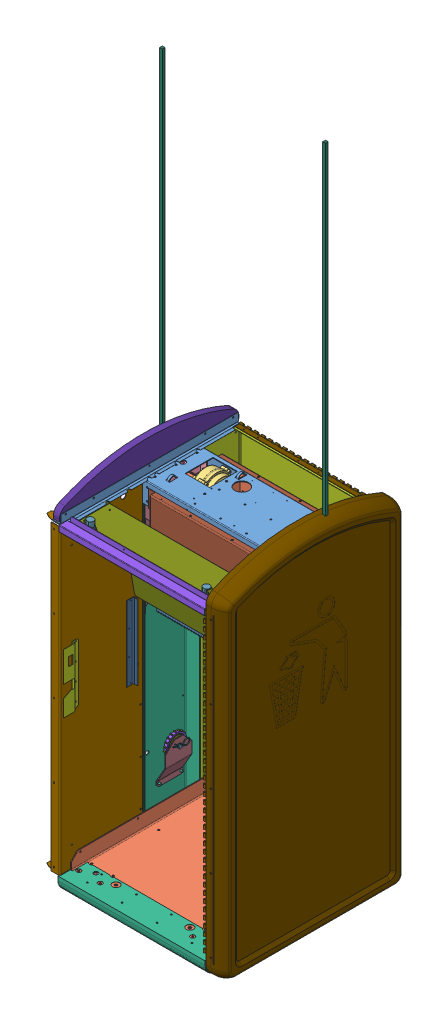
SolidWorks assembly BB3_Assy_Meca_3D_2, configuration Défaut. Lengths in mm.
Overall size (675.82 1282.03 663.93).
120 component instances, 56 part files, 9 mates.
Components (placement in the parent):
- BB3_Chassis-1: BB3_Chassis [Défaut] at (-140.0351 388.7943 -82.8142) size (675.82 1282.03 663.93)
  - TopCrossmember_Rev2-1: TopCrossmember_Rev2 [Default] at (20.5473 102.5902 0) size (635 86.99 210.82)
  - TopCrossMotorBrkt_Rev3-1: TopCrossMotorBrkt_Rev3 [Défaut] at (-101.9976 61.051 0) size (152.4 200.54 205.51)
  - Moto_Reducteur_011_562_1_216-1: Moto_Reducteur_011_562_1_216 [Default] at (192.9322 74.2423 -36.8146) x (0 -0.000019 -1) z (-1 0 0) size (114.3 226.4 239.81)
  - TopCrossBearingBrkt_Rev1-1: TopCrossBearingBrkt_Rev1 [Défaut] at (-246.0257 61.051 0) size (25.4 73.66 205.51)
  - TopCrossBearingBrkt_Rev1-2: TopCrossBearingBrkt_Rev1 [Défaut] at (287.1203 61.051 0) x (-1 0 0) z (0 0 -1) size (25.4 73.66 205.51)
  - Chassis_Coussinet-1: Chassis_Coussinet [Default] at (-247.5497 60.2788 -36.8146) x (0 -0.995993 0.089436) z (0 0.089436 0.995993) size (28.27 19.05 28.27)
  - Chassis_Coussinet-2: Chassis_Coussinet [Default] at (288.6443 60.2788 -36.8146) x (0 0.997938 0.064185) z (0 -0.064185 0.997938) size (28.27 19.05 28.27)
  - Chassis_Support_Moteur-1: Chassis_Support_Moteur [Défaut] at (-296.9017 100.6288 0.0002) x (0 0 1) z (0 1 0) size (205.51 54 1127)
  - Chassis_Support_Moteur-2: Chassis_Support_Moteur [Défaut] at (337.9963 100.6288 0.0002) x (0 0 -1) z (0 1 0) size (205.51 54 1127)
  - Chassis_Panneau_Arriere-2: Chassis_Panneau_Arriere [Défaut] at (20.5983 -479.4712 -246.619) x (0 0 1) z (0 1 0) size (164.98 667 1155.29)
  - Chassis_Support_Batterie-2: Chassis_Support_Batterie [Défaut] at (20.5983 -270.8192 -242.544) x (0 0 1) z (-1 0 0) size (116.32 446 529)
  - Chassis_Support_Moteur_Devant_Gauche-2: Chassis_Support_Moteur_Devant_Gauche [Défaut] at (-249.8894 -442.8187 130.7585) x (0 0 -1) z (0 1 0) size (329.85 66 1105)
  - Chassis_Positionnement_Emetteur_Recepteur_Gauche-2: Chassis_Positionnement_Emetteur_Recepteur_Gauche [Défaut] at (-222.4622 -381.8185 156.8606) x (1 0 0) z (0 -1 0) size (22.1 48.5 273)
  - Chassis_Support_Moteur_Devant_Droite-1: Chassis_Support_Moteur_Devant_Droite [Défaut] at (290.9839 -442.8187 130.7585) x (0 0 -1) z (0 -1 0) size (329.85 66 1105)
  - Chassis_Positionnement_Emetteur_Recepteur_Droite-1: Chassis_Positionnement_Emetteur_Recepteur_Droite [Défaut] at (263.5568 -381.8185 156.8606) x (-1 0 0) z (0 1 0) size (22.1 48.5 273)
  - Chassis_Support_Pignon_bas-1: Chassis_Support_Pignon_bas [Défaut] at (305.4963 -865.3715 -39.8528) x (-1 0 0) z (0 0 1) size (35.2 151.29 95)
  - Chassis_Axe_Pignon_Bas-1: Chassis_Axe_Pignon_Bas [Défaut] at (340.9963 -816.3715 -39.8528) x (-1 0 0) z (0 -0.052233 -0.998635) size (48.6 15.9 15.9)
  - Chassis_Goupille_Axe_Pignon_bas-1: Chassis_Goupille_Axe_Pignon_bas [Défaut] at (300.5463 -817.6251 -63.8201) x (0 0.052233 0.998635) z (1 0 0) size (60.5 23 3)
  - Chassis_Support_Pignon_bas-2: Chassis_Support_Pignon_bas [Défaut] at (-264.4017 -865.3715 -39.8528) x (1 0 0) z (0 0 -1) size (35.2 151.29 95)
  - Chassis_Axe_Pignon_Bas-2: Chassis_Axe_Pignon_Bas [Défaut] at (-299.9017 -816.3715 -39.8528) x (1 0 0) z (0 0.31653 0.948583) size (48.6 15.9 15.9)
  - Chassis_Goupille_Axe_Pignon_bas-2: Chassis_Goupille_Axe_Pignon_bas [Défaut] at (-259.4517 -808.7748 -17.0869) x (0 -0.31653 -0.948583) z (1 0 0) size (60.5 23 3)
  - Chassis_Plaque_Haute-1: Chassis_Plaque_Haute [Défaut] at (20.4963 92.768 412.6062) x (0 0 -1) z (1 0 0) size (278.51 354.1 562.7)
  - Chassis_Renfort-1: Chassis_Renfort [Défaut] at (20.5463 -1018.8712 0.0002) x (0 0 1) z (-1 0 0) size (199.51 39 641)
  - Chassis_Charniere_Photovoltaique-1: Chassis_Charniere_Photovoltaique [Défaut] at (20.5983 134.4053 -220.1468) x (0 0 -1) z (1 0 0) size (21.77 6 520)
  - Chassis_Equerre_Haute-1: Chassis_Equerre_Haute [Défaut] at (-246.1446 112.2812 81.6782) x (1 0 0.000001) z (-0.000001 0 1) size (44 37.45 648)
  - Chassis_Equerre_Haute-2: Chassis_Equerre_Haute [Défaut] at (287.2893 112.2812 81.6751) x (-1 0 -0.000168) z (0.000168 0 -1) size (44 37.45 648)
  - Chassis_Repose_Bac_Dechets-1: Chassis_Repose_Bac_Dechets [Défaut] at (20.4963 -992.8728 80.2436) x (0 -0.000001 1) z (-1 0 0) size (641.73 77 529)
  - Chassis_Semelle-1: Chassis_Semelle [Défaut] at (20.4963 -1034.3925 80.4561) x (1 0 0) z (0 -0.000001 1) size (404.15 56 558)
  - Chassis_Repose_Pied-1: Chassis_Repose_Pied [Défaut] at (-187.0037 -1049.3185 336.4561) x (1 0 0) z (0 -0.000001 1) size (94 52.5 63.3)
  - Chassis_Repose_Pied-2: Chassis_Repose_Pied [Défaut] at (-187.0037 -1049.3182 -175.5439) x (1 0 0) z (0 -0.000001 1) size (94 52.5 63.3)
  - Chassis_Repose_Pied-3: Chassis_Repose_Pied [Défaut] at (227.9963 -1049.3182 -175.5439) x (1 0 0) z (0 -0.000001 1) size (94 52.5 63.3)
  - Chassis_Repose_Pied-4: Chassis_Repose_Pied [Défaut] at (227.9963 -1049.3185 336.4561) x (1 0 0) z (0 -0.000001 1) size (94 52.5 63.3)
  - Chassis_Repose_Pied_Insert-1: Chassis_Repose_Pied_Insert [Défaut] at (-187.0037 -1050.3185 336.4561) x (0 1 0.000001) z (0.428959 -0.000001 0.903324) size (14.3 17.5 17.5)
  - Chassis_Repose_Pied_Insert-2: Chassis_Repose_Pied_Insert [Défaut] at (227.9963 -1050.3185 336.4561) x (0 1 0.000001) z (0.384049 -0.000001 0.923313) size (14.3 17.5 17.5)
  - Chassis_Repose_Pied_Insert-3: Chassis_Repose_Pied_Insert [Défaut] at (227.9963 -1050.3182 -175.5439) x (0 1 0.000001) z (-0.000001 -0.000001 1) size (14.3 17.5 17.5)
  - Chassis_Repose_Pied_Insert-4: Chassis_Repose_Pied_Insert [Défaut] at (-187.0037 -1050.3182 -175.5439) x (0 1 0.000001) z (-0.000001 -0.000001 1) size (14.3 17.5 17.5)
  - Chassis_Repose_Pied_Insert-5: Chassis_Repose_Pied_Insert [Défaut] at (-114.0037 -995.8185 336.4561) x (0 -1 -0.000001) z (0.798225 0 0.602359) size (14.3 17.5 17.5)
  - Chassis_Repose_Pied_Insert-6: Chassis_Repose_Pied_Insert [Défaut] at (154.9963 -995.8185 336.4561) x (0 -1 -0.000001) z (0.000001 -0.000001 1) size (14.3 17.5 17.5)
  - Chassis_Repose_Pied_Insert-7: Chassis_Repose_Pied_Insert [Défaut] at (-114.0037 -995.8182 -175.5439) x (0 -1 -0.000001) z (0.000001 -0.000001 1) size (14.3 17.5 17.5)
  - Chassis_Repose_Pied_Insert-8: Chassis_Repose_Pied_Insert [Défaut] at (154.9963 -995.8182 -175.5439) x (0 -1 -0.000001) z (0.000001 -0.000001 1) size (14.3 17.5 17.5)
  - Chassis_Dessous_Avant_Porte-1: Chassis_Dessous_Avant_Porte [Défaut] at (20.4963 -992.8728 80.2436) x (0 -0.000001 1) z (-1 0 0) size (98 53.79 536)
  - Chassis_Serrure-1: Chassis_Serrure [Défaut] at (-243.4017 -382.964 366.4072) x (1 0 0) z (0 1 0) size (10.5 63.82 216)
  - Chassis_Equerre_Face-1: Chassis_Equerre_Face [Défaut] at (20.4963 111.0096 411.9878) x (0 0 1) z (-1 0 0) size (32.2 41.42 529)
  - Chassis_Charniere_Support_Moteur_Devant_Droite-1: Chassis_Charniere_Support_Moteur_Devant_Droite [Défaut] at (260.2718 -465.3185 388.412) x (0 0 1) z (0 -1 0) size (21.77 6 1066)
  - Chassis_Serrure_Cle-1: Chassis_Serrure_Cle [Défaut] at (-191.3537 126.1269 363.7894) x (0 1 0) z (-1 0 0) size (41.58 38.56 38.97)
    - Chassis_Serrure_Came-1: Chassis_Serrure_Came [Défaut] at (-18.246 14.5659 16.3878) x (0 -1 0) z (1 0 0) size (12.45 12.01 13.54)
    - Chassis_Serrure_Rondelle_Ecrou-1: Chassis_Serrure_Rondelle_Ecrou [Défaut] at (-31.074 17.7899 -9.8703) x (0 0.096744 0.995309) z (-1 0 0) size (35.31 35.31 0.64)
    - Chassis_Serrure_Ecrou_Hex-1: Chassis_Serrure_Ecrou_Hex [Défaut] at (-26.3115 -31.157 8.2014) x (0 0 1) z (-1 0 0) size (33 28.58 4.76)
    - Chassis_Serrure_Insert_Cle-1: Chassis_Serrure_Insert_Cle [Défaut] at (26.379 -212.8643 14.6) x (-1 0 0) z (0 0 -1) size (23.33 15.95 15.95)
    - Chassis_Serrure_Support-1: Chassis_Serrure_Support [Défaut] at (-26.6815 11.1833 12.473) x (-1 0 0) z (0 -1 0) size (41.46 28.7 28.7)
    - Chassis_Serrure_Ressort-1: Chassis_Serrure_Ressort [Défaut] at (-1.4058 10.243 9.1044) x (0 0 -1) z (1 0 0) size (21.49 4.59 4.57)
    - Chassis_Serrure_Pene-1: Chassis_Serrure_Pene [Défaut] at (1.0072 5.2825 -10.1896) x (0 -0.999973 -0.007317) z (-1 0 0) size (16.91 23.47 9.63)
  - Chassis_Serrure_Cle-2: Chassis_Serrure_Cle [Défaut] at (232.3463 126.1269 341.4229) x (0 1 0) z (1 0 0) size (41.58 38.56 38.97)
    - Chassis_Serrure_Came-1: Chassis_Serrure_Came [Défaut] at (-18.246 14.5659 16.3878) x (0 -1 0) z (1 0 0) size (12.45 12.01 13.54)
    - Chassis_Serrure_Rondelle_Ecrou-1: Chassis_Serrure_Rondelle_Ecrou [Défaut] at (-31.074 17.7899 -9.8703) x (0 0.096744 0.995309) z (-1 0 0) size (35.31 35.31 0.64)
    - Chassis_Serrure_Ecrou_Hex-1: Chassis_Serrure_Ecrou_Hex [Défaut] at (-26.3115 -31.157 8.2014) x (0 0 1) z (-1 0 0) size (33 28.58 4.76)
    - Chassis_Serrure_Insert_Cle-1: Chassis_Serrure_Insert_Cle [Défaut] at (26.379 -212.8643 14.6) x (-1 0 0) z (0 0 -1) size (23.33 15.95 15.95)
    - Chassis_Serrure_Support-1: Chassis_Serrure_Support [Défaut] at (-26.6815 11.1833 12.473) x (-1 0 0) z (0 -1 0) size (41.46 28.7 28.7)
    - Chassis_Serrure_Ressort-1: Chassis_Serrure_Ressort [Défaut] at (-1.4058 10.243 9.1044) x (0 0 -1) z (1 0 0) size (21.49 4.59 4.57)
    - Chassis_Serrure_Pene-1: Chassis_Serrure_Pene [Défaut] at (1.0072 5.2825 -10.1896) x (0 -0.999973 -0.007317) z (-1 0 0) size (16.91 23.47 9.63)
  - Tombstone_Rev1-1: Tombstone_Rev1 [Default] at (288.5894 129.5652 81.0473) x (1 0 0.000168) z (-0.000168 0 1) size (22.23 105.62 654.05)
  - Tombstone_Rev1-2: Tombstone_Rev1 [Default] at (-247.4446 129.5652 82.3062) x (-1 0 -0.000001) z (0.000001 0 -1) size (22.23 105.62 654.05)
  - SideSkin_Rev1-1: SideSkin_Rev1 [Default] at (-317.3073 -1045.6118 82.3061) x (-1 0 -0.000001) z (0.000001 0 -1) size (69.87 1274.83 660.4) (hidden)
  - SideSkin_Rev1-2: SideSkin_Rev1 [Default] at (358.4521 -1045.6118 81.059) x (1 0 0.000168) z (-0.000168 0 1) size (69.87 1274.83 660.4)
  - Chassis_Interieur_Cache_Chaine-1: Chassis_Interieur_Cache_Chaine [Défaut] at (-242.9017 -763.8184 0) x (0 -0.000001 1) z (-1 0 0) size (249 989 21) (hidden)
  - Chassis_Interieur_Cache_Chaine-2: Chassis_Interieur_Cache_Chaine [Défaut] at (283.9963 -763.8185 0.0002) x (0 0 -1) z (1 0 0) size (249 989 21)
  - Chassis_Bac_Dechets-1: Chassis_Bac_Dechets [Défaut] at (19.5983 -711.9931 65.1059) x (-1 0 0) z (0 0.000001 -1) size (517 387.96 620.45) (hidden)
- BB3_Axe_Moteur-1: BB3_Axe_Moteur [Défaut] at (-118.6236 449.4588 -117.6952) size (601.11 82.55 82.55)
  - TransmissionShaft_Rev1-1: TransmissionShaft_Rev1 [Défaut] at (-0.7672 -0.3857 -1.9336) size (596.9 18.75 19.05)
  - CounterDisc_Rev1-1: CounterDisc_Rev1 [Défaut] at (188.8209 -0.3857 -1.9336) size (0.91 82.55 82.55)
  - Pignon_Haut-1: Pignon_Haut [Défaut] at (-297.0312 -0.3857 -1.9336) x (0 0 1) z (-1 0 0) (suppressed, hidden)
  - Pignon_Haut-2: Pignon_Haut [Défaut] at (294.0828 -0.3857 -1.9336) x (0 0 -1) z (1 0 0) (suppressed, hidden)
  - SHAFT_COLLAR_MCMASTER_6166K28-1: SHAFT_COLLAR_MCMASTER_6166K28 [Défaut] at (181.6772 -0.3857 -1.9336) size (14.29 38.1 38.1)
  - TRANSMISSION_KEY_MC_98870A140-1: TRANSMISSION_KEY_MC_98870A140 [Défaut] at (-285.8172 18.6654 -1.9336) x (-1 0 0) z (0 0 1) size (25.4 4.76 4.76)
  - TRANSMISSION_KEY_MC_98870A140-2: TRANSMISSION_KEY_MC_98870A140 [Défaut] at (284.2828 18.6654 -1.9336) x (-1 0 0) z (0 0 1) size (25.4 4.76 4.76)
  - TRANSMISSION_KEY_MC_98870A190-1: TRANSMISSION_KEY_MC_98870A190 [Défaut] at (-155.0672 18.6654 -1.9336) x (-1 0 0) z (0 0 1) size (63.5 4.76 4.76)
  - PURPLE_IGUS-1: PURPLE_IGUS [Défaut] at (191.2568 -0.3857 -1.9336) x (0 0.381849 -0.924225) z (0 0.924225 0.381849) size (28.27 19.05 28.27)
  - BB3_Pignon_Cylindre_Primitif-1: BB3_Pignon_Cylindre_Primitif [Défaut] at (-295.6312 -0.3857 -1.9336) x (0 0 -1) z (1 0 0) size (73.14 73.14 10)
  - BB3_Pignon_Cylindre_Primitif-2: BB3_Pignon_Cylindre_Primitif [Défaut] at (295.4828 -0.3857 -1.9336) x (0 0 -1) z (1 0 0) size (73.14 73.14 10)
  - Pignon_Haut-3: Pignon_Haut [Défaut] at (-297.0312 -0.3857 -1.9336) x (0 0 1) z (-1 0 0)
  - Pignon_Haut-4: Pignon_Haut [Défaut] at (296.8828 -0.3857 -1.9336) x (0 0 -1) z (1 0 0)
- BB3_Rame_Compacteur-1: BB3_Rame_Compacteur [Défaut] at (-143.8198 251.6092 -80.1568) size (627.3 1739.7 268.31)
  - Compacteur_Rame-1: Compacteur_Rame [Défaut] at (24.383 25.4321 -2.9042) size (505.8 287.44 265.81)
  - Compacteur_Flasque-1: Compacteur_Flasque [Défaut] at (23.883 58.9321 129.5958) x (-1 0 0) z (0 0 -1) size (481.4 343 21.8)
  - Compacteur_Flasque-2: Compacteur_Flasque [Défaut] at (24.883 58.9321 -135.4042) size (481.4 343 21.8)
  - Compacteur_Guide_Droit-1: Compacteur_Guide_Droit [Défaut] at (297.583 154.6611 -2.9042) x (0 0 1) z (0 -1 0) size (185.61 92.3 356)
  - Compacteur_Guide_Gauche-1: Compacteur_Guide_Gauche [Défaut] at (-250.117 154.6611 -2.9042) x (0 0 -1) z (0 -1 0) size (185.61 93.6 356)
  - Compacteur_Guide_Patin-1: Compacteur_Guide_Patin [Défaut] at (-270.917 -23.3389 -95.7102) x (-1 0 0) z (0 0 -1) size (38 350 6.7)
  - Compacteur_Guide_Patin-2: Compacteur_Guide_Patin [Défaut] at (-270.917 -23.3389 89.9018) size (38 350 6.7)
  - Compacteur_Guide_Patin-3: Compacteur_Guide_Patin [Défaut] at (318.383 -23.3389 89.9018) size (38 350 6.7)
  - Compacteur_Guide_Patin-4: Compacteur_Guide_Patin [Défaut] at (318.383 -23.3389 -95.7102) x (-1 0 0) z (0 0 -1) size (38 350 6.7)
  - BB3_Coulissant_Vertical_Cremaillere-1: BB3_Coulissant_Vertical_Cremaillere [Défaut] at (-273.2835 838.3611 2.0958) x (-1 0 0) z (0 -1 0) size (10 10 1400)
  - BB3_Coulissant_Vertical_Cremaillere-2: BB3_Coulissant_Vertical_Cremaillere [Défaut] at (320.7496 838.3611 2.0958) x (1 0 0) z (0 1 0) size (10 10 1400)
- BB3_Pignon_Bas-1: BB3_Pignon_Bas [Défaut] at (-415.6548 -432.9543 -114.7035) x (0 0 -1) z (1 0 0) size (78.63 79.65 18.29)
  - Pignon_Bas-1: Pignon_Bas [Défaut] at (7.9635 5.3771 0) size (78.63 79.65 11.2)
  - Bearing_203KRR5-1: Bearing_203KRR5 [Défaut] at (7.9635 5.3771 0) x (0 0 -1) z (1 0 0) size (12 56.49 56.49)
    - Bearing_203KRR5_BE-1: Bearing_203KRR5_BE [Défaut] x (-1 0 0) z (0 -0.669852 0.742494) size (12 40 40)
    - Bearing_203KRR5_ER-1: Bearing_203KRR5_ER [Défaut] at (0 10.8207 9.7621) x (1 0 0) z (0 0.742494 0.669852) size (6 6 6)
    - Bearing_203KRR5_ER-2: Bearing_203KRR5_ER [Défaut] at (0 14.3789 -2.3734) x (1 0 0) z (0 0.986649 -0.162859) size (6 6 6)
    - Bearing_203KRR5_ER-3: Bearing_203KRR5_ER [Défaut] at (0 7.1095 -12.7217) x (1 0 0) z (0 0.487837 -0.872935) size (6 6 6)
    - Bearing_203KRR5_ER-4: Bearing_203KRR5_ER [Défaut] at (0 -5.5135 -13.4903) x (1 0 0) z (0 -0.378326 -0.925672) size (6 6 6)
    - Bearing_203KRR5_ER-5: Bearing_203KRR5_ER [Défaut] at (0 -13.9848 -4.1004) x (1 0 0) z (0 -0.959602 -0.28136) size (6 6 6)
    - Bearing_203KRR5_ER-6: Bearing_203KRR5_ER [Défaut] at (0 -11.9252 8.3772) x (1 0 0) z (0 -0.818278 0.574822) size (6 6 6)
    - Bearing_203KRR5_ER-7: Bearing_203KRR5_ER [Défaut] at (0 -0.8857 14.5466) x (1 0 0) z (0 -0.060774 0.998152) size (6 6 6)
  - Bearing_203KRR5_BI-1: Bearing_203KRR5_BI [Défaut] at (7.9635 5.3771 0) x (0 0 -1) z (1 0 0) size (18.29 24.43 24.43)
  - BB3_Pignon_Cylindre_Primitif-1: BB3_Pignon_Cylindre_Primitif [Défaut] at (7.9635 5.3771 1.4) size (73.14 73.14 10)
- BB3_Pignon_Bas-2: BB3_Pignon_Bas [Défaut] at (178.2592 -432.9543 -130.6306) x (0 0 1) z (-1 0 0) size (78.63 79.65 18.29)
  - Pignon_Bas-1: Pignon_Bas [Défaut] at (7.9635 5.3771 0) size (78.63 79.65 11.2)
  - Bearing_203KRR5-1: Bearing_203KRR5 [Défaut] at (7.9635 5.3771 0) x (0 0 -1) z (1 0 0) size (12 56.49 56.49)
    - Bearing_203KRR5_BE-1: Bearing_203KRR5_BE [Défaut] x (-1 0 0) z (0 -0.669852 0.742494) size (12 40 40)
    - Bearing_203KRR5_ER-1: Bearing_203KRR5_ER [Défaut] at (0 10.8207 9.7621) x (1 0 0) z (0 0.742494 0.669852) size (6 6 6)
    - Bearing_203KRR5_ER-2: Bearing_203KRR5_ER [Défaut] at (0 14.3789 -2.3734) x (1 0 0) z (0 0.986649 -0.162859) size (6 6 6)
    - Bearing_203KRR5_ER-3: Bearing_203KRR5_ER [Défaut] at (0 7.1095 -12.7217) x (1 0 0) z (0 0.487837 -0.872935) size (6 6 6)
    - Bearing_203KRR5_ER-4: Bearing_203KRR5_ER [Défaut] at (0 -5.5135 -13.4903) x (1 0 0) z (0 -0.378326 -0.925672) size (6 6 6)
    - Bearing_203KRR5_ER-5: Bearing_203KRR5_ER [Défaut] at (0 -13.9848 -4.1004) x (1 0 0) z (0 -0.959602 -0.28136) size (6 6 6)
    - Bearing_203KRR5_ER-6: Bearing_203KRR5_ER [Défaut] at (0 -11.9252 8.3772) x (1 0 0) z (0 -0.818278 0.574822) size (6 6 6)
    - Bearing_203KRR5_ER-7: Bearing_203KRR5_ER [Défaut] at (0 -0.8857 14.5466) x (1 0 0) z (0 -0.060774 0.998152) size (6 6 6)
  - Bearing_203KRR5_BI-1: Bearing_203KRR5_BI [Défaut] at (7.9635 5.3771 0) x (0 0 -1) z (1 0 0) size (18.29 24.43 24.43)
  - BB3_Pignon_Cylindre_Primitif-1: BB3_Pignon_Cylindre_Primitif [Défaut] at (7.9635 5.3771 1.4) size (73.14 73.14 10)
Mates (geometry in assembly coordinates):
- Coaxiale1: concentric anti-aligned: cylinder of BB3_Chassis-1/Chassis_Coussinet-1 through (-387.5848 449.0731 -119.6288) axis (1 0 0) radius 9.6139; cylinder of BB3_Axe_Moteur-1/TransmissionShaft_Rev1-1 through (179.0592 449.0731 -119.6288) axis (-1 0 0) radius 9.525
- Distance1: distance = 9.56 mm anti-aligned: plane of BB3_Axe_Moteur-1/Pignon_Haut-3 through (-397.1448 449.0731 -119.6288) normal (1 0 0); plane of BB3_Chassis-1/Chassis_Coussinet-1 through (-387.5848 449.0731 -119.6288) normal (-1 0 0)
- Coïncidente2: coincident aligned: plane of BB3_Chassis-1/Chassis_Panneau_Arriere-2; plane of BB3_Rame_Compacteur-1/Compacteur_Rame-1 through (-119.4368 277.0413 -83.061) normal (1 0 0)
- Coïncidente3: coincident anti-aligned: plane of BB3_Chassis-1/Chassis_Support_Moteur-1 through (-385.9368 -637.5769 -182.567) normal (0 0 1); plane of BB3_Rame_Compacteur-1/Compacteur_Guide_Patin-1 through (-414.7368 228.2703 -182.567) normal (0 0 -1)
- Distance2: distance = 12 mm aligned: plane of BB3_Rame_Compacteur-1/Compacteur_Flasque-2 through (-335.4368 482.0413 -215.561) normal (0 1 0); plane of BB3_Chassis-1/TopCrossmember_Rev2-1 through (-436.9878 494.0413 22.5958) normal (0 1 0)
- Coaxiale2: concentric anti-aligned: cylinder of BB3_Chassis-1/Chassis_Axe_Pignon_Bas-2 through (-417.6368 -427.5772 -122.667) axis (1 0 0) radius 6.25; cylinder of BB3_Pignon_Bas-1/Bearing_203KRR5_BI-1 through (-415.6548 -427.5772 -122.667) axis (-1 0 0) radius 6.5405
- Coïncidente5: coincident aligned: plane of BB3_Axe_Moteur-1/Pignon_Haut-3 through (-419.2548 469.8587 -119.6288) normal (-1 0 0); plane of BB3_Pignon_Bas-1/Pignon_Bas-1 through (-419.2548 -406.7916 -122.667) normal (-1 0 0)
- Coaxiale3: concentric anti-aligned: cylinder of BB3_Chassis-1/Chassis_Axe_Pignon_Bas-1 through (178.6612 -427.5772 -122.667) axis (-1 0 0) radius 6.25; cylinder of BB3_Pignon_Bas-2/Bearing_203KRR5_BI-1 through (178.2592 -427.5772 -122.667) axis (1 0 0) radius 6.5405
- Coïncidente6: coincident aligned: plane of BB3_Axe_Moteur-1/Pignon_Haut-4 through (181.8592 469.8587 -119.6288) normal (1 0 0); plane of BB3_Pignon_Bas-2/Pignon_Bas-1 through (181.8592 -406.7916 -122.667) normal (1 0 0)
